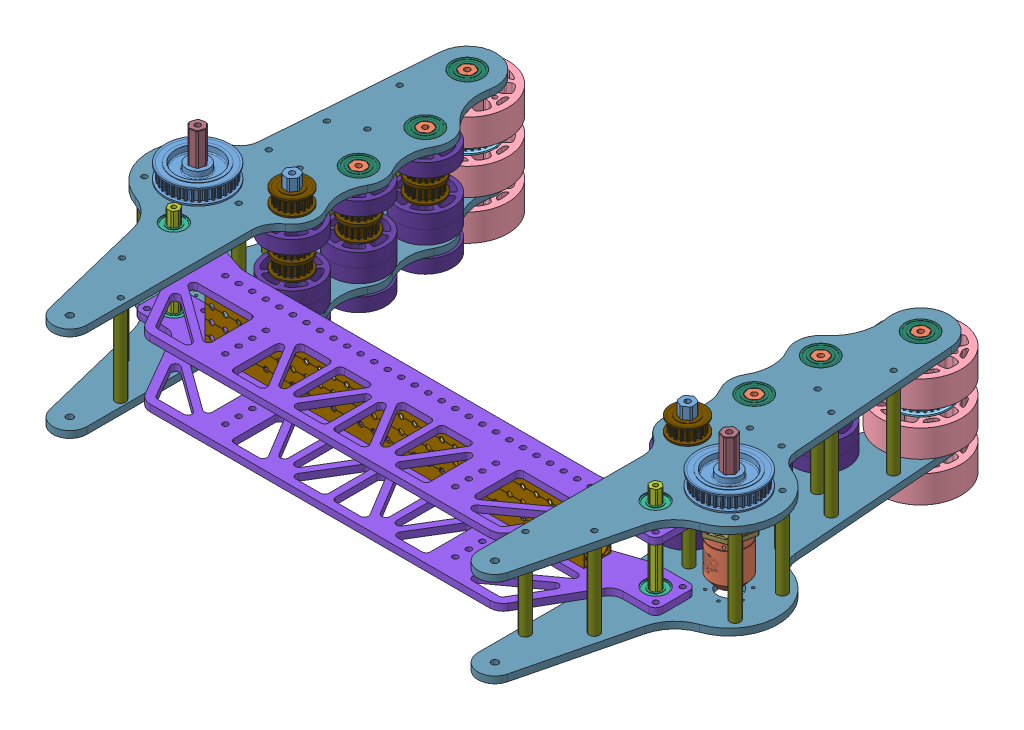
SolidWorks assembly Roller Claw, configuration Default. Lengths in mm.
Overall size (590.37 159.05 455.23).
163 component instances, 27 part files, 12 mates.
Components (placement in the parent):
- Right Roller Claw-1: Right Roller Claw [Default] at (339.7553 150.3563 318.0728) size (145.49 159.05 454.48)
  - 36T_HTD_5mmP_9mmW_flanged_500_hex_217-3231-1: 36T_HTD_5mmP_9mmW_flanged_500_hex_217-3231 [Default] at (179.6545 359.9234 345.8295) x (-0.337159 0 -0.941448) z (0 -1 0) size (60 60 14.5)
  - ultraplanetary-1: ultraplanetary [Default] at (198.2743 320.0734 349.6112) x (-0.199034 0 0.979992) z (0 -1 0) size (63.81 63.81 121.86)
    - REV-21-1651-1: REV-21-1651 [Default] at (0 19 -11.5) x (0 0 1) z (-0.999972 -0.007497 0) size (56.01 42.91 43.01)
    - REV-41-1601-1: REV-41-1601 [Default] at (0 19 -10) x (-0.5 -0.866025 0) z (0 0 1) size (43.62 38.42 17.88)
    - REV-41-1604-1: REV-41-1604 [Default] at (0 19 -26.25) x (-0.5 0.866025 0) z (0 0 1) size (54.69 56.73 18.25)
      - REV-41-1604.STEP-1: REV-41-1604.STEP [Default] at origin size (54.69 56.73 18.25)
        - REV-41-1604-2.STEP-1: REV-41-1604-2.STEP [Default] at origin size (43.57 38 6.25)
        - REV-41-1604-1.STEP-1: REV-41-1604-1.STEP [Default] at (0 0 7) x (0.5 0.866025 0) z (0 0 -1) size (43.57 38 7.03)
        - 6704ZZ.STEP-1: 6704ZZ.STEP [Default] at (0 0 7.75) x (0.995 -0.099871 0) z (0 0 1) size (27 27 4)
        - 6704ZZ.STEP-2: 6704ZZ.STEP [Default] at (0 0 3) x (0.993119 0.117109 0) z (0 0 1) size (27 27 4)
        - REV-40-1606_Through Hole.STEP-1: REV-40-1606_Through Hole.STEP [Default] at (0 0 10.95) x (-0.517794 -0.855505 0) z (0 0 -1) size (22 22 16.95)
        - REV-41-1604-4.STEP-1: REV-41-1604-4.STEP [Default] at (0 0 9.7) x (0.517794 0.855505 0) z (0 0 1) size (22 22 1.25)
        - REV-41-1604-3.STEP-1: REV-41-1604-3.STEP [Default] at (0 0 5) size (27.02 27 1.12)
        - socket head cap screw_am_B18.3.1M - 2 x 0.4 x 4 Hex SHCS -- 4NHX.STEP-1: socket head cap screw_am_B18.3.1M - 2 x 0.4 x 4 Hex SHCS -- 4NHX.STEP [Default] at (-11.8435 -10.7579 11.2) x (0 0 -1) z (-0.492915 -0.870077 0) size (6 3.8 3.8)
        - socket head cap screw_am_B18.3.1M - 2 x 0.4 x 4 Hex SHCS -- 4NHX.STEP-2: socket head cap screw_am_B18.3.1M - 2 x 0.4 x 4 Hex SHCS -- 4NHX.STEP [Default] at (-3.3948 15.6357 11.2) x (0 0 -1) z (-0.934724 -0.355374 0) size (6 3.8 3.8)
        - socket head cap screw_am_B18.3.1M - 2 x 0.4 x 4 Hex SHCS -- 4NHX.STEP-3: socket head cap screw_am_B18.3.1M - 2 x 0.4 x 4 Hex SHCS -- 4NHX.STEP [Default] at (15.2383 -4.8778 11.2) x (0 0 -1) z (0.970727 -0.240185 0) size (6 3.8 3.8)
        - 91294A003_BLACK ALLOY STEEL FLAT-HEAD SOCKET CAP SCREW_91294A003.STEP-1: 91294A003_BLACK ALLOY STEEL FLAT-HEAD SOCKET CAP SCREW_91294A003.STEP [Default] at (6.5084 3.5803 10.95) size (4 4 5)
        - 91294A003_BLACK ALLOY STEEL FLAT-HEAD SOCKET CAP SCREW_91294A003.STEP-2: 91294A003_BLACK ALLOY STEEL FLAT-HEAD SOCKET CAP SCREW_91294A003.STEP [Default] at (-0.1535 -7.4266 10.95) size (4 4 5)
        - 91294A003_BLACK ALLOY STEEL FLAT-HEAD SOCKET CAP SCREW_91294A003.STEP-3: 91294A003_BLACK ALLOY STEEL FLAT-HEAD SOCKET CAP SCREW_91294A003.STEP [Default] at (-6.3549 3.8463 10.95) size (4 4 5)
    - REV-41-1607-1: REV-41-1607 [Default] at (0 19 0) x (-1 0 0) z (0 -1 0) size (43.57 5 38.01)
    - REV-41-1620-1: REV-41-1620 [Default] at (0 19 -32.25) x (0.876175 0.481992 0) z (0 0 1) size (22 22 46.85)
  - Claw Plates-2: Claw Plates [Default] at (-69.8106 346.3234 416.9495) size (132.77 6.35 429.09)
  - thunderhex_flanged_217-4006-10: thunderhex_flanged_217-4006 [Default] at (115.7867 348.7046 321.0569) x (0.592492 0 0.805576) z (0 -1 0) size (31.12 31.12 7.94)
  - thunderhex_flanged_217-4006-11: thunderhex_flanged_217-4006 [Default] at (115.7867 348.7046 258.5475) x (-0.906539 0 -0.422123) z (0 -1 0) size (31.12 31.12 7.94)
  - thunderhex_flanged_217-4006-12: thunderhex_flanged_217-4006 [Default] at (115.7867 348.7046 196.0381) x (-0.994435 0 -0.105355) z (0 -1 0) size (31.12 31.12 7.94)
  - thunderhex_flanged_217-4006-13: thunderhex_flanged_217-4006 [Default] at (142.9222 348.7046 129.5022) x (0.097157 0 0.995269) z (0 -1 0) size (31.12 31.12 7.94)
  - Claw Plates-1: Claw Plates [Default] at (-69.8106 263.7734 416.9495) size (132.77 6.35 429.09)
  - thunderhex_flanged_217-4006-1: thunderhex_flanged_217-4006 [Default] at (115.7867 267.7421 321.0569) x (0.900767 0 -0.434303) z (0 1 0) size (31.12 31.12 7.94)
  - thunderhex_flanged_217-4006-3: thunderhex_flanged_217-4006 [Default] at (115.7867 267.7421 258.5475) x (-0.989804 0 -0.142438) z (0 1 0) size (31.12 31.12 7.94)
  - thunderhex_flanged_217-4006-4: thunderhex_flanged_217-4006 [Default] at (115.7867 267.7421 196.0381) x (-0.890133 0 -0.4557) z (0 1 0) size (31.12 31.12 7.94)
  - thunderhex_flanged_217-4006-5: thunderhex_flanged_217-4006 [Default] at (142.9222 267.7421 129.5022) x (-0.890133 0 -0.4557) z (0 1 0) size (31.12 31.12 7.94)
  - 3_000_L_10_thru_WCP-0209-1: 3_000_L_10_thru_WCP-0209 [Default] at (120.1277 308.2234 477.6333) x (0 1 0) z (-0.241352 0 0.970438) size (76.2 9.5 9.5)
  - 3_000_L_10_thru_WCP-0209-2: 3_000_L_10_thru_WCP-0209 [Default] at (151.8777 308.2234 444.6133) x (0 1 0) z (-0.241352 0 0.970438) size (76.2 9.5 9.5)
  - 3_000_L_10_thru_WCP-0209-3: 3_000_L_10_thru_WCP-0209 [Default] at (141.5239 308.2234 345.4022) x (0 1 0) z (-0.241352 0 0.970438) size (76.2 9.5 9.5)
  - 3_000_L_10_thru_WCP-0209-4: 3_000_L_10_thru_WCP-0209 [Default] at (207.4135 308.2234 368.0545) x (0 1 0) z (-0.241352 0 0.970438) size (76.2 9.5 9.5)
  - 3_000_L_10_thru_WCP-0209-5: 3_000_L_10_thru_WCP-0209 [Default] at (207.4135 308.2234 323.6045) x (0 -1 0) z (-0.328723 0 0.944426) size (76.2 9.5 9.5)
  - 3_000_L_10_thru_WCP-0209-6: 3_000_L_10_thru_WCP-0209 [Default] at (170.8852 308.2234 287.9041) x (0 1 0) z (-0.241352 0 0.970438) size (76.2 9.5 9.5)
  - 3_000_L_10_thru_WCP-0209-7: 3_000_L_10_thru_WCP-0209 [Default] at (141.5239 308.2234 288.2522) x (0 1 0) z (-0.241352 0 0.970438) size (76.2 9.5 9.5)
  - 3_000_L_10_thru_WCP-0209-8: 3_000_L_10_thru_WCP-0209 [Default] at (166.9239 308.2234 237.2588) x (0 1 0) z (-0.241352 0 0.970438) size (76.2 9.5 9.5)
  - 3_000_L_10_thru_WCP-0209-9: 3_000_L_10_thru_WCP-0209 [Default] at (141.5239 308.2234 224.7522) x (0 1 0) z (-0.241352 0 0.970438) size (76.2 9.5 9.5)
  - 3_000_L_10_thru_WCP-0209-10: 3_000_L_10_thru_WCP-0209 [Default] at (161.9722 308.2234 173.9522) x (0 1 0) z (-0.241352 0 0.970438) size (76.2 9.5 9.5)
  - 2_OD_30A_Straight_Flex_Wheel_217-6353-1: 2_OD_30A_Straight_Flex_Wheel_217-6353 [Default] at (115.7867 293.7234 321.0569) x (-0.99292 0 0.118786) z (0.118786 0 0.99292) size (50.8 12.7 50.8)
  - 18T_HTD_5mmP_9mmW_flanged_500_hex_217-3225-2: 18T_HTD_5mmP_9mmW_flanged_500_hex_217-3225 [Default] at (115.7867 307.3234 321.0569) x (-0.800501 0 0.599331) z (0 -1 0) size (32 32 14.5)
  - 18T_HTD_5mmP_9mmW_flanged_500_hex_217-3225-1: 18T_HTD_5mmP_9mmW_flanged_500_hex_217-3225 [Default] at (115.7867 321.8234 321.0569) x (-0.800501 0 0.599331) z (0 1 0) size (32 32 14.5)
  - 2_OD_30A_Straight_Flex_Wheel_217-6353-3: 2_OD_30A_Straight_Flex_Wheel_217-6353 [Default] at (115.7867 335.4234 321.0569) x (-0.99292 0 0.118786) z (0.118786 0 0.99292) size (50.8 12.7 50.8)
  - 2_OD_30A_Straight_Flex_Wheel_217-6353-2: 2_OD_30A_Straight_Flex_Wheel_217-6353 [Default] at (115.7867 281.0234 321.0569) x (-0.99292 0 0.118786) z (0.118786 0 0.99292) size (50.8 12.7 50.8)
  - 2_OD_30A_Straight_Flex_Wheel_217-6353-13: 2_OD_30A_Straight_Flex_Wheel_217-6353 [Default] at (115.7867 257.4234 321.0569) x (-0.99292 0 0.118786) z (0.118786 0 0.99292) size (50.8 12.7 50.8)
  - 1_2thunderhex_5.5in-1: 1_2thunderhex_5.5in [Default] at (115.7867 695.5734 321.0569) x (-0.919287 0 -0.393589) z (0 -1 0) size (13.74 12.75 139.7)
  - 18T_HTD_5mmP_9mmW_flanged_500_hex_217-3225-9: 18T_HTD_5mmP_9mmW_flanged_500_hex_217-3225 [Default] at (115.7867 359.9234 321.0569) x (-0.800501 0 0.599331) z (0 -1 0) size (32 32 14.5)
  - 2_OD_30A_Straight_Flex_Wheel_217-6353-7: 2_OD_30A_Straight_Flex_Wheel_217-6353 [Default] at (115.7867 293.7234 258.5475) x (-0.956763 0 0.290869) z (0.290869 0 0.956763) size (50.8 12.7 50.8)
  - 18T_HTD_5mmP_9mmW_flanged_500_hex_217-3225-5: 18T_HTD_5mmP_9mmW_flanged_500_hex_217-3225 [Default] at (115.7867 307.3234 258.5475) x (-0.683146 0 0.730282) z (0 -1 0) size (32 32 14.5)
  - 18T_HTD_5mmP_9mmW_flanged_500_hex_217-3225-6: 18T_HTD_5mmP_9mmW_flanged_500_hex_217-3225 [Default] at (115.7867 321.8234 258.5475) x (-0.683146 0 0.730282) z (0 1 0) size (32 32 14.5)
  - 2_OD_30A_Straight_Flex_Wheel_217-6353-8: 2_OD_30A_Straight_Flex_Wheel_217-6353 [Default] at (115.7867 335.4234 258.5475) x (-0.956763 0 0.290869) z (0.290869 0 0.956763) size (50.8 12.7 50.8)
  - 2_OD_30A_Straight_Flex_Wheel_217-6353-9: 2_OD_30A_Straight_Flex_Wheel_217-6353 [Default] at (115.7867 281.0234 258.5475) x (-0.956763 0 0.290869) z (0.290869 0 0.956763) size (50.8 12.7 50.8)
  - 1_2thunderhex_4.5in-2: 1_2thunderhex_4.5in [Default] at (115.7867 695.5734 258.5475) x (0.683146 0 -0.730282) z (0 -1 0) size (13.74 12.75 114.3)
  - 2_OD_30A_Straight_Flex_Wheel_217-6353-14: 2_OD_30A_Straight_Flex_Wheel_217-6353 [Default] at (115.7867 257.4234 258.5475) x (-0.730282 0 -0.683146) z (-0.683146 0 0.730282) size (50.8 12.7 50.8)
  - 2_OD_30A_Straight_Flex_Wheel_217-6353-10: 2_OD_30A_Straight_Flex_Wheel_217-6353 [Default] at (115.7867 293.7234 196.0381) x (0.94551 0 -0.325593) z (-0.325593 0 -0.94551) size (50.8 12.7 50.8)
  - 18T_HTD_5mmP_9mmW_flanged_500_hex_217-3225-7: 18T_HTD_5mmP_9mmW_flanged_500_hex_217-3225 [Default] at (115.7867 307.3234 196.0381) x (0.656039 0 -0.754727) z (0 -1 0) size (32 32 14.5)
  - 18T_HTD_5mmP_9mmW_flanged_500_hex_217-3225-8: 18T_HTD_5mmP_9mmW_flanged_500_hex_217-3225 [Default] at (115.7867 321.8234 196.0381) x (0.656039 0 -0.754727) z (0 1 0) size (32 32 14.5)
  - 2_OD_30A_Straight_Flex_Wheel_217-6353-11: 2_OD_30A_Straight_Flex_Wheel_217-6353 [Default] at (115.7867 335.4234 196.0381) x (0.94551 0 -0.325593) z (-0.325593 0 -0.94551) size (50.8 12.7 50.8)
  - 2_OD_30A_Straight_Flex_Wheel_217-6353-12: 2_OD_30A_Straight_Flex_Wheel_217-6353 [Default] at (115.7867 281.0234 196.0381) x (0.94551 0 -0.325593) z (-0.325593 0 -0.94551) size (50.8 12.7 50.8)
  - 1_2thunderhex_4.5in-3: 1_2thunderhex_4.5in [Default] at (115.7867 695.5734 196.0381) x (0.656039 0 -0.754727) z (0 -1 0) size (13.74 12.75 114.3)
  - 2_OD_30A_Straight_Flex_Wheel_217-6353-15: 2_OD_30A_Straight_Flex_Wheel_217-6353 [Default] at (115.7867 257.4234 196.0381) x (-0.190783 0 0.981632) z (0.981632 0 0.190783) size (50.8 12.7 50.8)
  - wide_roller_wheel-1: wide_roller_wheel [Default] at (123.4101 254.2514 114.098) x (-0.521403 0 0.853311) z (-0.853311 0 -0.521403) size (76.2 25.4 76.2)
    - wide_wheel_mount-1: wide_wheel_mount [Default] at (2.9708 21.322 -24.6817) size (28.57 25.4 28.57)
    - 3_OD_30A_Straight_Flex_Wheel-1: 3_OD_30A_Straight_Flex_Wheel [Default] at (2.9708 34.022 -24.6817) size (76.2 25.4 76.2)
  - wide_roller_wheel-2: wide_roller_wheel [Default] at (123.4101 294.1514 114.098) x (-0.521403 0 0.853311) z (-0.853311 0 -0.521403) size (76.2 25.4 76.2)
    - wide_wheel_mount-1: wide_wheel_mount [Default] at (2.9708 21.322 -24.6817) size (28.57 25.4 28.57)
    - 3_OD_30A_Straight_Flex_Wheel-1: 3_OD_30A_Straight_Flex_Wheel [Default] at (2.9708 34.022 -24.6817) size (76.2 25.4 76.2)
  - 30T_HTD_5mmP_9mmW_flanged_500_hex_217-3229-2: 30T_HTD_5mmP_9mmW_flanged_500_hex_217-3229 [Default] at (142.9222 308.2234 129.5022) x (0.521403 0 -0.853311) z (0 1 0) size (51 51 14.5)
  - 1_2thunderhex_4.5in-4: 1_2thunderhex_4.5in [Default] at (142.9222 695.5734 129.5022) x (-0.99969 0 -0.024892) z (0 -1 0) size (13.74 12.75 114.3)
  - wide_roller_wheel-3: wide_roller_wheel [Default] at (162.4344 217.0514 144.9063) x (0.521403 0 -0.853311) z (0.853311 0 0.521403) size (76.2 25.4 76.2)
    - wide_wheel_mount-1: wide_wheel_mount [Default] at (2.9708 21.322 -24.6817) size (28.57 25.4 28.57)
    - 3_OD_30A_Straight_Flex_Wheel-1: 3_OD_30A_Straight_Flex_Wheel [Default] at (2.9708 34.022 -24.6817) size (76.2 25.4 76.2)
  - thunderhex_375_flanged_217-5829-1: thunderhex_375_flanged_217-5829 [Default] at (156.2494 344.7359 391.5495) x (0 1 0) z (-0.397184 0 0.917739) size (7.11 24.61 24.61)
  - thunderhex_375_flanged_217-5829-2: thunderhex_375_flanged_217-5829 [Default] at (156.2494 271.7109 391.5495) x (0 -1 0) z (0 0 1) size (7.11 24.61 24.61)
  - 3_8thunderhex_4.5in-1: 3_8thunderhex_4.5in [Default] at (156.2494 -91.8266 391.5495) x (0.142102 0 -0.989852) z (0 -1 0) size (10.24 9.53 114.3)
  - thunderhex_375_flanged_217-5829-3: thunderhex_375_flanged_217-5829 [Default] at (156.2494 274.8859 391.5495) x (0 1 0) z (0.329672 0 -0.944096) size (7.11 24.61 24.61)
  - thunderhex_375_flanged_217-5829-4: thunderhex_375_flanged_217-5829 [Default] at (156.2494 341.5609 391.5495) x (0 -1 0) z (0.640533 0 0.76793) size (7.11 24.61 24.61)
- Left Roller Claw-1: Left Roller Claw [Default] at (-161.3847 238.4838 416.2723) size (145.24 159.05 455.23)
  - 36T_HTD_5mmP_9mmW_flanged_500_hex_217-3231-1: 36T_HTD_5mmP_9mmW_flanged_500_hex_217-3231 [Default] at (181.8644 271.7959 247.63) x (0.29796 0 -0.954578) z (0 -1 0) size (60 60 14.5)
  - ultraplanetary-1: ultraplanetary [Default] at (194.4494 231.9459 261.8645) x (-0.749181 0 0.662365) z (0 -1 0) size (63.81 63.81 121.86)
    - REV-21-1651-1: REV-21-1651 [Default] at (0 19 -11.5) x (0 0 1) z (-0.999972 -0.007497 0) size (56.01 42.91 43.01)
    - REV-41-1601-1: REV-41-1601 [Default] at (0 19 -10) x (-0.5 -0.866025 0) z (0 0 1) size (43.62 38.42 17.88)
    - REV-41-1604-1: REV-41-1604 [Default] at (0 19 -26.25) x (-0.5 0.866025 0) z (0 0 1) size (54.69 56.73 18.25)
      - REV-41-1604.STEP-1: REV-41-1604.STEP [Default] at origin size (54.69 56.73 18.25)
        - REV-41-1604-2.STEP-1: REV-41-1604-2.STEP [Default] at origin size (43.57 38 6.25)
        - REV-41-1604-1.STEP-1: REV-41-1604-1.STEP [Default] at (0 0 7) x (0.5 0.866025 0) z (0 0 -1) size (43.57 38 7.03)
        - 6704ZZ.STEP-1: 6704ZZ.STEP [Default] at (0 0 7.75) x (0.995 -0.099871 0) z (0 0 1) size (27 27 4)
        - 6704ZZ.STEP-2: 6704ZZ.STEP [Default] at (0 0 3) x (0.993119 0.117109 0) z (0 0 1) size (27 27 4)
        - REV-40-1606_Through Hole.STEP-1: REV-40-1606_Through Hole.STEP [Default] at (0 0 10.95) x (-0.517794 -0.855505 0) z (0 0 -1) size (22 22 16.95)
        - REV-41-1604-4.STEP-1: REV-41-1604-4.STEP [Default] at (0 0 9.7) x (0.517794 0.855505 0) z (0 0 1) size (22 22 1.25)
        - REV-41-1604-3.STEP-1: REV-41-1604-3.STEP [Default] at (0 0 5) size (27.02 27 1.12)
        - socket head cap screw_am_B18.3.1M - 2 x 0.4 x 4 Hex SHCS -- 4NHX.STEP-1: socket head cap screw_am_B18.3.1M - 2 x 0.4 x 4 Hex SHCS -- 4NHX.STEP [Default] at (-11.8435 -10.7579 11.2) x (0 0 -1) z (-0.492915 -0.870077 0) size (6 3.8 3.8)
        - socket head cap screw_am_B18.3.1M - 2 x 0.4 x 4 Hex SHCS -- 4NHX.STEP-2: socket head cap screw_am_B18.3.1M - 2 x 0.4 x 4 Hex SHCS -- 4NHX.STEP [Default] at (-3.3948 15.6357 11.2) x (0 0 -1) z (-0.934724 -0.355374 0) size (6 3.8 3.8)
        - socket head cap screw_am_B18.3.1M - 2 x 0.4 x 4 Hex SHCS -- 4NHX.STEP-3: socket head cap screw_am_B18.3.1M - 2 x 0.4 x 4 Hex SHCS -- 4NHX.STEP [Default] at (15.2383 -4.8778 11.2) x (0 0 -1) z (0.970727 -0.240185 0) size (6 3.8 3.8)
        - 91294A003_BLACK ALLOY STEEL FLAT-HEAD SOCKET CAP SCREW_91294A003.STEP-1: 91294A003_BLACK ALLOY STEEL FLAT-HEAD SOCKET CAP SCREW_91294A003.STEP [Default] at (6.5084 3.5803 10.95) size (4 4 5)
        - 91294A003_BLACK ALLOY STEEL FLAT-HEAD SOCKET CAP SCREW_91294A003.STEP-2: 91294A003_BLACK ALLOY STEEL FLAT-HEAD SOCKET CAP SCREW_91294A003.STEP [Default] at (-0.1535 -7.4266 10.95) size (4 4 5)
        - 91294A003_BLACK ALLOY STEEL FLAT-HEAD SOCKET CAP SCREW_91294A003.STEP-3: 91294A003_BLACK ALLOY STEEL FLAT-HEAD SOCKET CAP SCREW_91294A003.STEP [Default] at (-6.3549 3.8463 10.95) size (4 4 5)
    - REV-41-1607-1: REV-41-1607 [Default] at (0 19 0) x (-1 0 0) z (0 -1 0) size (43.57 5 38.01)
    - REV-41-1620-1: REV-41-1620 [Default] at (0 19 -32.25) x (0.876175 0.481992 0) z (0 0 1) size (22 22 46.85)
  - Claw Plates-2: Claw Plates [Default] at (431.3295 264.5459 318.75) x (-1 0 0) z (0 0 1) size (132.77 6.35 429.09)
  - thunderhex_flanged_217-4006-10: thunderhex_flanged_217-4006 [Default] at (245.7322 260.5771 222.8574) x (0.592492 0 0.805576) z (0 -1 0) size (31.12 31.12 7.94)
  - thunderhex_flanged_217-4006-11: thunderhex_flanged_217-4006 [Default] at (245.7322 260.5771 160.348) x (-0.906539 0 -0.422123) z (0 -1 0) size (31.12 31.12 7.94)
  - thunderhex_flanged_217-4006-12: thunderhex_flanged_217-4006 [Default] at (245.7322 260.5771 97.8386) x (-0.881857 0 -0.471518) z (0 -1 0) size (31.12 31.12 7.94)
  - thunderhex_flanged_217-4006-13: thunderhex_flanged_217-4006 [Default] at (218.5967 260.5771 31.3027) x (0.097157 0 0.995269) z (0 -1 0) size (31.12 31.12 7.94)
  - Claw Plates-1: Claw Plates [Default] at (431.3295 181.9959 318.75) x (-1 0 0) z (0 0 1) size (132.77 6.35 429.09)
  - thunderhex_flanged_217-4006-1: thunderhex_flanged_217-4006 [Default] at (245.7322 179.6146 222.8574) x (0.900767 0 -0.434303) z (0 1 0) size (31.12 31.12 7.94)
  - thunderhex_flanged_217-4006-3: thunderhex_flanged_217-4006 [Default] at (245.7322 179.6146 160.348) x (-0.989504 0 -0.144504) z (0 1 0) size (31.12 31.12 7.94)
  - thunderhex_flanged_217-4006-4: thunderhex_flanged_217-4006 [Default] at (245.7322 179.6146 97.8386) x (-0.243579 0 -0.969881) z (0 1 0) size (31.12 31.12 7.94)
  - thunderhex_flanged_217-4006-5: thunderhex_flanged_217-4006 [Default] at (218.5967 179.6146 31.3027) x (-0.890339 0 -0.455299) z (0 1 0) size (31.12 31.12 7.94)
  - 3_000_L_10_thru_WCP-0209-1: 3_000_L_10_thru_WCP-0209 [Default] at (219.995 220.0959 247.2027) x (0 1 0) z (-0.241352 0 0.970438) size (76.2 9.5 9.5)
  - 3_000_L_10_thru_WCP-0209-2: 3_000_L_10_thru_WCP-0209 [Default] at (241.3912 220.0959 379.4338) x (0 1 0) z (-0.241352 0 0.970438) size (76.2 9.5 9.5)
  - 3_000_L_10_thru_WCP-0209-3: 3_000_L_10_thru_WCP-0209 [Default] at (154.1054 220.0959 225.405) x (0 1 0) z (-0.241352 0 0.970438) size (76.2 9.5 9.5)
  - 3_000_L_10_thru_WCP-0209-4: 3_000_L_10_thru_WCP-0209 [Default] at (209.6412 220.0959 346.4138) x (0 1 0) z (-0.241352 0 0.970438) size (76.2 9.5 9.5)
  - 3_000_L_10_thru_WCP-0209-5: 3_000_L_10_thru_WCP-0209 [Default] at (154.1054 220.0959 269.855) x (0 -1 0) z (-0.328723 0 0.944426) size (76.2 9.5 9.5)
  - 3_000_L_10_thru_WCP-0209-6: 3_000_L_10_thru_WCP-0209 [Default] at (190.6337 220.0959 189.7046) x (0 1 0) z (-0.241352 0 0.970438) size (76.2 9.5 9.5)
  - 3_000_L_10_thru_WCP-0209-7: 3_000_L_10_thru_WCP-0209 [Default] at (219.995 220.0959 190.0527) x (0 1 0) z (-0.241352 0 0.970438) size (76.2 9.5 9.5)
  - 3_000_L_10_thru_WCP-0209-8: 3_000_L_10_thru_WCP-0209 [Default] at (194.595 220.0959 139.0593) x (0 1 0) z (-0.241352 0 0.970438) size (76.2 9.5 9.5)
  - 3_000_L_10_thru_WCP-0209-9: 3_000_L_10_thru_WCP-0209 [Default] at (219.995 220.0959 126.5527) x (0 1 0) z (-0.241352 0 0.970438) size (76.2 9.5 9.5)
  - 3_000_L_10_thru_WCP-0209-10: 3_000_L_10_thru_WCP-0209 [Default] at (199.5467 220.0959 75.7527) x (0 -1 0) z (0.241352 0 0.970438) size (76.2 9.5 9.5)
  - 2_OD_30A_Straight_Flex_Wheel_217-6353-1: 2_OD_30A_Straight_Flex_Wheel_217-6353 [Default] at (245.7322 205.5959 222.8574) x (0.111174 0 -0.993801) z (-0.993801 0 -0.111174) size (50.8 12.7 50.8)
  - 18T_HTD_5mmP_9mmW_flanged_500_hex_217-3225-2: 18T_HTD_5mmP_9mmW_flanged_500_hex_217-3225 [Default] at (245.7322 219.1959 222.8574) x (-0.400621 0 -0.916244) z (0 -1 0) size (32 32 14.5)
  - 18T_HTD_5mmP_9mmW_flanged_500_hex_217-3225-1: 18T_HTD_5mmP_9mmW_flanged_500_hex_217-3225 [Default] at (245.7322 233.6959 222.8574) x (-0.400621 0 -0.916244) z (0 1 0) size (32 32 14.5)
  - 2_OD_30A_Straight_Flex_Wheel_217-6353-3: 2_OD_30A_Straight_Flex_Wheel_217-6353 [Default] at (245.7322 247.2959 222.8574) x (0.111174 0 -0.993801) z (-0.993801 0 -0.111174) size (50.8 12.7 50.8)
  - 2_OD_30A_Straight_Flex_Wheel_217-6353-2: 2_OD_30A_Straight_Flex_Wheel_217-6353 [Default] at (245.7322 192.8959 222.8574) x (0.111174 0 -0.993801) z (-0.993801 0 -0.111174) size (50.8 12.7 50.8)
  - 2_OD_30A_Straight_Flex_Wheel_217-6353-13: 2_OD_30A_Straight_Flex_Wheel_217-6353 [Default] at (245.7322 169.2959 222.8574) x (0.111174 0 -0.993801) z (-0.993801 0 -0.111174) size (50.8 12.7 50.8)
  - 1_2thunderhex_5.5in-1: 1_2thunderhex_5.5in [Default] at (245.7322 607.4459 222.8574) x (0.59318 0 -0.80507) z (0 -1 0) size (13.74 12.75 139.7)
  - 18T_HTD_5mmP_9mmW_flanged_500_hex_217-3225-9: 18T_HTD_5mmP_9mmW_flanged_500_hex_217-3225 [Default] at (245.7322 271.7959 222.8574) x (-0.400621 0 -0.916244) z (0 -1 0) size (32 32 14.5)
  - 2_OD_30A_Straight_Flex_Wheel_217-6353-7: 2_OD_30A_Straight_Flex_Wheel_217-6353 [Default] at (245.7322 205.5959 160.348) x (0.996179 0 -0.087336) z (-0.087336 0 -0.996179) size (50.8 12.7 50.8)
  - 18T_HTD_5mmP_9mmW_flanged_500_hex_217-3225-5: 18T_HTD_5mmP_9mmW_flanged_500_hex_217-3225 [Default] at (245.7322 219.1959 160.348) x (0.819048 0 -0.573725) z (0 -1 0) size (32 32 14.5)
  - 18T_HTD_5mmP_9mmW_flanged_500_hex_217-3225-6: 18T_HTD_5mmP_9mmW_flanged_500_hex_217-3225 [Default] at (245.7322 233.6959 160.348) x (0.819048 0 -0.573725) z (0 1 0) size (32 32 14.5)
  - 2_OD_30A_Straight_Flex_Wheel_217-6353-8: 2_OD_30A_Straight_Flex_Wheel_217-6353 [Default] at (245.7322 247.2959 160.348) x (0.996179 0 -0.087336) z (-0.087336 0 -0.996179) size (50.8 12.7 50.8)
  - 2_OD_30A_Straight_Flex_Wheel_217-6353-9: 2_OD_30A_Straight_Flex_Wheel_217-6353 [Default] at (245.7322 192.8959 160.348) x (0.996179 0 -0.087336) z (-0.087336 0 -0.996179) size (50.8 12.7 50.8)
  - 1_2thunderhex_4.5in-2: 1_2thunderhex_4.5in [Default] at (245.7322 607.4459 160.348) x (-0.819048 0 0.573725) z (0 -1 0) size (13.74 12.75 114.3)
  - 2_OD_30A_Straight_Flex_Wheel_217-6353-14: 2_OD_30A_Straight_Flex_Wheel_217-6353 [Default] at (245.7322 169.2959 160.348) x (0.573725 0 0.819048) z (0.819048 0 -0.573725) size (50.8 12.7 50.8)
  - 2_OD_30A_Straight_Flex_Wheel_217-6353-10: 2_OD_30A_Straight_Flex_Wheel_217-6353 [Default] at (245.7322 205.5959 97.8386) x (0.37446 0 -0.927243) z (-0.927243 0 -0.37446) size (50.8 12.7 50.8)
  - 18T_HTD_5mmP_9mmW_flanged_500_hex_217-3225-7: 18T_HTD_5mmP_9mmW_flanged_500_hex_217-3225 [Default] at (245.7322 219.1959 97.8386) x (-0.139329 0 -0.990246) z (0 -1 0) size (32 32 14.5)
  - 18T_HTD_5mmP_9mmW_flanged_500_hex_217-3225-8: 18T_HTD_5mmP_9mmW_flanged_500_hex_217-3225 [Default] at (245.7322 233.6959 97.8386) x (-0.139329 0 -0.990246) z (0 1 0) size (32 32 14.5)
  - 2_OD_30A_Straight_Flex_Wheel_217-6353-11: 2_OD_30A_Straight_Flex_Wheel_217-6353 [Default] at (245.7322 247.2959 97.8386) x (0.37446 0 -0.927243) z (-0.927243 0 -0.37446) size (50.8 12.7 50.8)
  - 2_OD_30A_Straight_Flex_Wheel_217-6353-12: 2_OD_30A_Straight_Flex_Wheel_217-6353 [Default] at (245.7322 192.8959 97.8386) x (0.37446 0 -0.927243) z (-0.927243 0 -0.37446) size (50.8 12.7 50.8)
  - 1_2thunderhex_4.5in-3: 1_2thunderhex_4.5in [Default] at (245.7322 607.4459 97.8386) x (-0.139329 0 -0.990246) z (0 -1 0) size (13.74 12.75 114.3)
  - 2_OD_30A_Straight_Flex_Wheel_217-6353-15: 2_OD_30A_Straight_Flex_Wheel_217-6353 [Default] at (245.7322 169.2959 97.8386) x (0.615786 0 0.787914) z (0.787914 0 -0.615786) size (50.8 12.7 50.8)
  - wide_roller_wheel-1: wide_roller_wheel [Default] at (230.4702 166.1239 53.1437) x (0.815195 0 -0.579187) z (0.579187 0 0.815195) size (76.2 25.4 76.2)
    - wide_wheel_mount-1: wide_wheel_mount [Default] at (2.9708 21.322 -24.6817) size (28.57 25.4 28.57)
    - 3_OD_30A_Straight_Flex_Wheel-1: 3_OD_30A_Straight_Flex_Wheel [Default] at (2.9708 34.022 -24.6817) size (76.2 25.4 76.2)
  - wide_roller_wheel-2: wide_roller_wheel [Default] at (230.4702 206.0239 53.1437) x (0.815195 0 -0.579187) z (0.579187 0 0.815195) size (76.2 25.4 76.2)
    - wide_wheel_mount-1: wide_wheel_mount [Default] at (2.9708 21.322 -24.6817) size (28.57 25.4 28.57)
    - 3_OD_30A_Straight_Flex_Wheel-1: 3_OD_30A_Straight_Flex_Wheel [Default] at (2.9708 34.022 -24.6817) size (76.2 25.4 76.2)
  - 30T_HTD_5mmP_9mmW_flanged_500_hex_217-3229-2: 30T_HTD_5mmP_9mmW_flanged_500_hex_217-3229 [Default] at (218.5967 220.0959 31.3027) x (-0.815195 0 0.579187) z (0 1 0) size (51 51 14.5)
  - 1_2thunderhex_4.5in-4: 1_2thunderhex_4.5in [Default] at (218.5967 607.4459 31.3027) x (0.815195 0 -0.579187) z (0 -1 0) size (13.74 12.75 114.3)
  - wide_roller_wheel-3: wide_roller_wheel [Default] at (193.745 128.9239 30.6649) x (0.093993 0 0.995573) z (-0.995573 0 0.093993) size (76.2 25.4 76.2)
    - wide_wheel_mount-1: wide_wheel_mount [Default] at (2.9708 21.322 -24.6817) size (28.57 25.4 28.57)
    - 3_OD_30A_Straight_Flex_Wheel-1: 3_OD_30A_Straight_Flex_Wheel [Default] at (2.9708 34.022 -24.6817) size (76.2 25.4 76.2)
  - thunderhex_375_flanged_217-5829-1: thunderhex_375_flanged_217-5829 [Default] at (205.2695 253.4334 293.35) x (0 -1 0) z (-0.936737 0 0.350033) size (7.11 24.61 24.61)
  - thunderhex_375_flanged_217-5829-2: thunderhex_375_flanged_217-5829 [Default] at (205.2695 186.7584 293.35) x (0 1 0) z (-0.988109 0 -0.153752) size (7.11 24.61 24.61)
  - 3_8thunderhex_4.5in-1: 3_8thunderhex_4.5in [Default] at (205.2695 -179.9541 293.35) x (0.998853 0 -0.047878) z (0 -1 0) size (10.24 9.53 114.3)
  - thunderhex_375_flanged_217-5829-3: thunderhex_375_flanged_217-5829 [Default] at (205.2695 183.5834 293.35) x (0 -1 0) z (-0.263366 0 0.964696) size (7.11 24.61 24.61)
  - thunderhex_375_flanged_217-5829-4: thunderhex_375_flanged_217-5829 [Default] at (205.2695 256.6084 293.35) x (0 1 0) z (-0.521845 0 0.85304) size (7.11 24.61 24.61)
- Part52-1: Part52 [Default] at (269.9447 483.9797 735.0223) x (1 0 0) z (0 1 0) size (490.22 107.95 6.35)
- Part52-2: Part52 [Default] at (269.9447 426.8297 735.0223) x (1 0 0) z (0 1 0) size (490.22 107.95 6.35)
- 14inTube-1: 14inTube [Default] at (1241.4947 458.5797 715.9723) x (0 0 -1) z (1 0 0) size (25.4 50.8 355.6)
Mates (geometry in assembly coordinates):
- Coincident1: coincident aligned: plane of Right Roller Claw-1/Claw Plates-2 through (412.6722 503.0297 461.8074) normal (0 1 0); plane of Left Roller Claw-1/Claw Plates-2 through (127.2173 503.0297 461.8074) normal (0 1 0)
- Parallel1: parallel anti-aligned: plane of Right Roller Claw-1/Claw Plates-2 through (453.533 503.0297 679.236) normal (-1 0 0); plane of Left Roller Claw-1/Claw Plates-2 through (86.3565 496.6797 679.236) normal (1 0 0)
- Coincident14: coincident anti-aligned: plane of Left Roller Claw-1/thunderhex_375_flanged_217-5829-1 through (47.7745 490.3297 720.0318) normal (0 -1 0); plane of Part52-1 through (269.9447 490.3297 735.0223) normal (0 1 0)
- Concentric8: concentric anti-aligned: cylinder of Right Roller Claw-1/thunderhex_375_flanged_217-5829-4 through (496.0047 491.9172 709.6223) axis (0 1 0) radius 11.1125; cylinder of Part52-1 through (496.0047 490.3297 709.6223) axis (0 -1 0) radius 11.1125
- Concentric11: concentric anti-aligned: cylinder of Left Roller Claw-1/thunderhex_375_flanged_217-5829-1 through (43.8847 491.9172 709.6223) axis (0 1 0) radius 11.1125; cylinder of Part52-1 through (43.8847 490.3297 709.6223) axis (0 -1 0) radius 11.1125
- Parallel6: parallel aligned: plane of Part52-1 through (269.9447 490.3297 728.6723) normal (0 0 1)
- Concentric12: concentric aligned: cylinder of Left Roller Claw-1/thunderhex_375_flanged_217-5829-2 through (43.8847 425.2422 709.6223) axis (0 -1 0) radius 11.1125; cylinder of Part52-2 through (43.8847 433.1797 709.6223) axis (0 -1 0) radius 11.1125
- Coincident16: coincident anti-aligned: plane of Left Roller Claw-1/thunderhex_375_flanged_217-5829-2 through (45.5933 426.8297 698.6419) normal (0 1 0); plane of Part52-2 through (269.9447 426.8297 735.0223) normal (0 -1 0)
- Concentric13: concentric aligned: cylinder of Right Roller Claw-1/thunderhex_375_flanged_217-5829-3 through (496.0047 425.2422 709.6223) axis (0 -1 0) radius 11.1125; cylinder of Part52-2 through (496.0047 433.1797 709.6223) axis (0 -1 0) radius 11.1125
- Coincident17: coincident anti-aligned: plane of Part52-1 through (269.9447 483.9797 735.0223) normal (0 -1 0); plane of 14inTube-1 through (60.3947 483.9797 703.2723) normal (0 1 0)
- Coincident18: coincident aligned: plane of Part52-1 through (269.9447 490.3297 703.2723) normal (0 0 -1); plane of 14inTube-1 through (60.3947 433.1797 703.2723) normal (0 0 -1)
- Concentric14: concentric anti-aligned: cylinder of Part52-1 through (441.3947 490.3297 715.9723) axis (0 -1 0) radius 2.54; cylinder of 14inTube-1 through (441.3947 433.1797 715.9723) axis (0 1 0) radius 2.5
